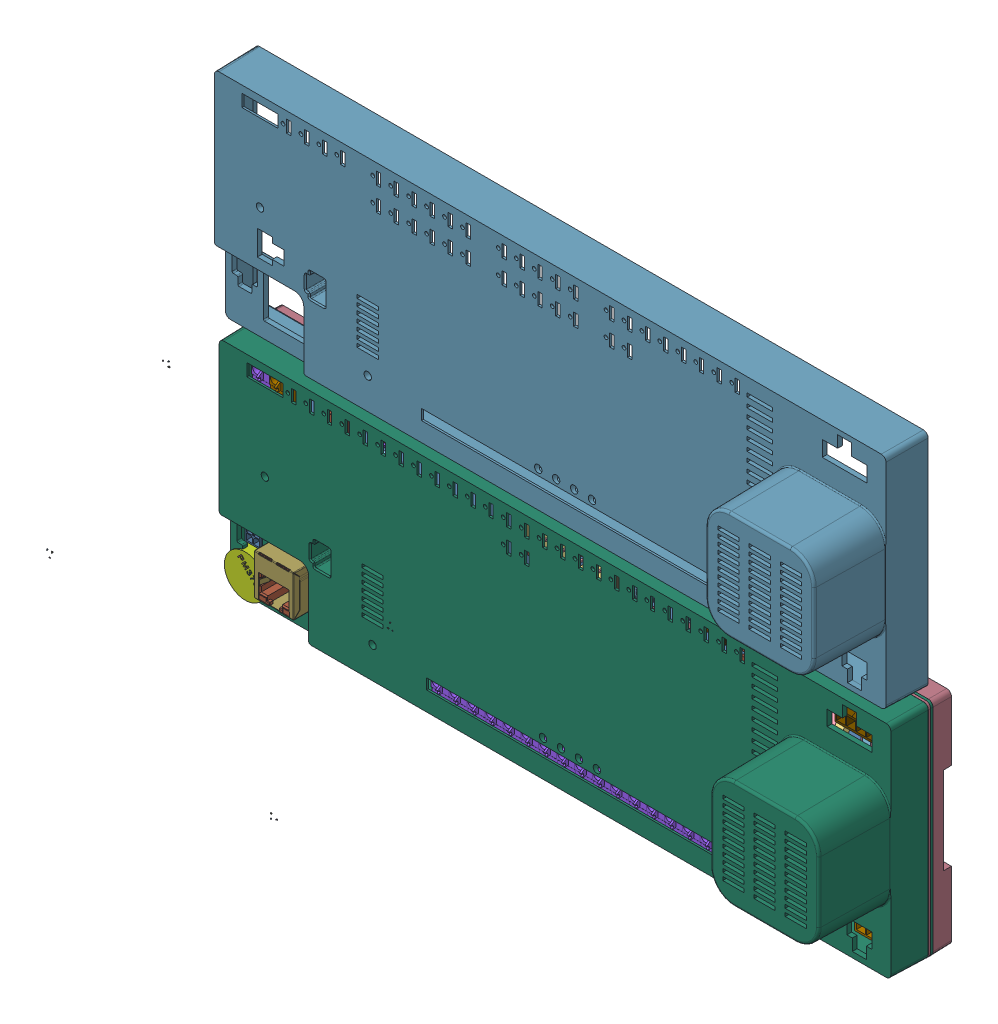
SolidWorks assembly _SC944D, configuration Default. Lengths in mm. (continued)
Components (placement in the parent): (continued)
- T58-1: T58 [Default] at origin size (130.97 33.9 23.48)
  - SW3dPS-transistor_SOT233-1: SW3dPS-transistor_SOT233 [Default] at (127.5968 31.0332 -21.9) x (-1 0 0) z (0 1 0) size (2.9 1.1 1.6)
  - SW3dPS-transistor_SOT233_1-1: SW3dPS-transistor_SOT233_1 [Default] at (0.1276 0.031 -0.0219) x (-1 0 0) z (0 1 0) size (2.18 2.18 2.18)
  - SW3dPS-transistor_SOT233_2-1: SW3dPS-transistor_SOT233_2 [Default] at (0.0001 0 0) x (-1 0 0) z (0 1 0) size (2.18 2.18 2.18)
  - SW3dPS-transistor_SOT233_3-1: SW3dPS-transistor_SOT233_3 [Default] x (-1 0 0) z (0 1 0) size (2.18 2.18 2.18)
- T59-1: T59 [Default] at origin size (136.17 33.9 23.48)
  - SW3dPS-transistor_SOT233-1: SW3dPS-transistor_SOT233 [Default] at (132.8038 31.0332 -21.9) x (-1 0 0) z (0 1 0) size (2.9 1.1 1.6)
  - SW3dPS-transistor_SOT233_1-1: SW3dPS-transistor_SOT233_1 [Default] at (0.1328 0.031 -0.0219) x (-1 0 0) z (0 1 0) size (2.18 2.18 2.18)
  - SW3dPS-transistor_SOT233_2-1: SW3dPS-transistor_SOT233_2 [Default] at (0.0001 0 0) x (-1 0 0) z (0 1 0) size (2.18 2.18 2.18)
  - SW3dPS-transistor_SOT233_3-1: SW3dPS-transistor_SOT233_3 [Default] x (-1 0 0) z (0 1 0) size (2.18 2.18 2.18)
- T60-1: T60 [Default] at origin size (90.38 86.77 23.48)
  - SW3dPS-transistor_SOT233-1: SW3dPS-transistor_SOT233 [Default] at (86.9062 83.9018 -21.9) x (1 0 0) z (0 -1 0) size (2.9 1.1 1.6)
  - SW3dPS-transistor_SOT233_1-1: SW3dPS-transistor_SOT233_1 [Default] at (0.0869 0.0839 -0.0219) x (1 0 0) z (0 -1 0) size (2.18 2.18 2.18)
  - SW3dPS-transistor_SOT233_2-1: SW3dPS-transistor_SOT233_2 [Default] at (0.0001 0.0001 0) x (1 0 0) z (0 -1 0) size (2.18 2.18 2.18)
  - SW3dPS-transistor_SOT233_3-1: SW3dPS-transistor_SOT233_3 [Default] x (1 0 0) z (0 -1 0) size (2.18 2.18 2.18)
- T61-1: T61 [Default] at origin size (89.91 93.6 23.48)
  - SW3dPS-transistor_SOT233-1: SW3dPS-transistor_SOT233 [Default] at (86.4299 90.7281 -21.9) x (1 0 0) z (0 -1 0) size (2.9 1.1 1.6)
  - SW3dPS-transistor_SOT233_1-1: SW3dPS-transistor_SOT233_1 [Default] at (0.0864 0.0907 -0.0219) x (1 0 0) z (0 -1 0) size (2.18 2.18 2.18)
  - SW3dPS-transistor_SOT233_2-1: SW3dPS-transistor_SOT233_2 [Default] at (0.0001 0.0001 0) x (1 0 0) z (0 -1 0) size (2.18 2.18 2.18)
  - SW3dPS-transistor_SOT233_3-1: SW3dPS-transistor_SOT233_3 [Default] x (1 0 0) z (0 -1 0) size (2.18 2.18 2.18)
- T62-1: T62 [Default] at origin size (81.97 92.65 23.48)
  - SW3dPS-transistor_SOT233-1: SW3dPS-transistor_SOT233 [Default] at (78.4924 89.7756 -21.9) x (1 0 0) z (0 -1 0) size (2.9 1.1 1.6)
  - SW3dPS-transistor_SOT233_1-1: SW3dPS-transistor_SOT233_1 [Default] at (0.0785 0.0898 -0.0219) x (1 0 0) z (0 -1 0) size (2.18 2.18 2.18)
  - SW3dPS-transistor_SOT233_2-1: SW3dPS-transistor_SOT233_2 [Default] at (0.0001 0.0001 0) x (1 0 0) z (0 -1 0) size (2.18 2.18 2.18)
  - SW3dPS-transistor_SOT233_3-1: SW3dPS-transistor_SOT233_3 [Default] x (1 0 0) z (0 -1 0) size (2.18 2.18 2.18)
- T63-1: T63 [Default] at origin size (84.51 85.66 23.48)
  - SW3dPS-transistor_SOT233-1: SW3dPS-transistor_SOT233 [Default] at (81.0324 82.7906 -21.9) x (1 0 0) z (0 -1 0) size (2.9 1.1 1.6)
  - SW3dPS-transistor_SOT233_1-1: SW3dPS-transistor_SOT233_1 [Default] at (0.081 0.0828 -0.0219) x (1 0 0) z (0 -1 0) size (2.18 2.18 2.18)
  - SW3dPS-transistor_SOT233_2-1: SW3dPS-transistor_SOT233_2 [Default] at (0.0001 0.0001 0) x (1 0 0) z (0 -1 0) size (2.18 2.18 2.18)
  - SW3dPS-transistor_SOT233_3-1: SW3dPS-transistor_SOT233_3 [Default] x (1 0 0) z (0 -1 0) size (2.18 2.18 2.18)
- T64-1: T64 [Default] at origin size (158.8 53.28 23.48)
  - SW3dPS-transistor_SOT233-1: SW3dPS-transistor_SOT233 [Default] at (155.3274 50.4056 -21.9) x (1 0 0) z (0 -1 0) size (2.9 1.1 1.6)
  - SW3dPS-transistor_SOT233_1-1: SW3dPS-transistor_SOT233_1 [Default] at (0.1553 0.0504 -0.0219) x (1 0 0) z (0 -1 0) size (2.18 2.18 2.18)
  - SW3dPS-transistor_SOT233_2-1: SW3dPS-transistor_SOT233_2 [Default] at (0.0002 0.0001 0) x (1 0 0) z (0 -1 0) size (2.18 2.18 2.18)
  - SW3dPS-transistor_SOT233_3-1: SW3dPS-transistor_SOT233_3 [Default] x (1 0 0) z (0 -1 0) size (2.18 2.18 2.18)
- T65-1: T65 [Default] at origin size (32.85 79.63 23.48)
  - SW3dPS-transistor_SOT233-1: SW3dPS-transistor_SOT233 [Default] at (29.9742 76.1522 -21.9) x (0 1 0) z (1 0 0) size (2.9 1.1 1.6)
  - SW3dPS-transistor_SOT233_1-1: SW3dPS-transistor_SOT233_1 [Default] at (0.03 0.0762 -0.0219) x (0 1 0) z (1 0 0) size (2.18 2.18 2.18)
  - SW3dPS-transistor_SOT233_2-1: SW3dPS-transistor_SOT233_2 [Default] at (0 0.0001 0) x (0 1 0) z (1 0 0) size (2.18 2.18 2.18)
  - SW3dPS-transistor_SOT233_3-1: SW3dPS-transistor_SOT233_3 [Default] x (0 1 0) z (1 0 0) size (2.18 2.18 2.18)
- T66-1: T66 [Default] at origin size (165.61 55.37 23.48)
  - SW3dPS-transistor_SOT233-1: SW3dPS-transistor_SOT233 [Default] at (162.2678 52.4962 -21.9) x (-1 0 0) z (0 1 0) size (2.9 1.1 1.6)
  - SW3dPS-transistor_SOT233_1-1: SW3dPS-transistor_SOT233_1 [Default] at (0.1623 0.0525 -0.0219) x (-1 0 0) z (0 1 0) size (2.18 2.18 2.18)
  - SW3dPS-transistor_SOT233_2-1: SW3dPS-transistor_SOT233_2 [Default] at (0.0002 0.0001 0) x (-1 0 0) z (0 1 0) size (2.18 2.18 2.18)
  - SW3dPS-transistor_SOT233_3-1: SW3dPS-transistor_SOT233_3 [Default] x (-1 0 0) z (0 1 0) size (2.18 2.18 2.18)
- U1-1: U1 [Default] at origin size (6.4 5 1.08)
  - SW3dPS-TSSOP-16-1: SW3dPS-TSSOP-16 [Default] at (33.8137 57.7851 0) x (0 1 0) z (0 0 1) size (5 6.4 1.08)
- U2-1: U2 [Default] at origin size (3 3 1.35)
  - User_Library-SOT23-6-1: User_Library-SOT23-6 [Default] at (72.8979 53.5939 0) x (-1 0 0) z (0 0 1) size (3 3 1.35)
- U3-1: U3 [Default] at origin size (9.19 5.08 4.7)
  - SOIC_pin_2-1: SOIC_pin_2 [Default] at (91.8173 23.0238 1) x (0 1 0) z (1 0 0) size (0.4 1.1 1.1)
  - SOIC_pin_2-2: SOIC_pin_2 [Default] at (88.8236 28.0938 1) x (0 -1 0) z (-1 0 0) size (0.4 1.1 1.1)
  - SOIC_pin_2-3: SOIC_pin_2 [Default] at (88.8236 30.6337 1) x (0 -1 0) z (-1 0 0) size (0.4 1.1 1.1)
  - SOIC_pin_2-4: SOIC_pin_2 [Default] at (91.8173 20.4838 1) x (0 1 0) z (1 0 0) size (0.4 1.1 1.1)
  - 1175074120-1: 1175074120 [Default] at (93.6466 25.5588 0) size (0.41 5.08 4.5)
    - Extruded-1: Extruded [Default] at origin size (0.41 5.08 4.5)
  - 1175073984-1: 1175073984 [Default] at (90.3287 25.5588 0) size (7.05 5.08 4.6)
    - Extruded_1-1: Extruded_1 [Default] at origin size (7.05 5.08 4.6)
  - 1173466944-1: 1173466944 [Default] at (92.2336 23.6538 4.6) x (0 1 0) z (0 0 1) size (0.4 0.4 0.1)
    - Cylinder-1: Cylinder [Default] at origin size (0.4 0.4 0.1)
- U4-1: U4 [Default] at origin size (19.5 9.8 14.1)
  - 1175074392-1: 1175074392 [Default] at (162.4959 50.1649 -1.6) size (0.5 0.5 1.6)
    - Extruded_2-1: Extruded_2 [Default] at origin size (0.5 0.5 1.6)
  - 1175074392-2: 1175074392 [Default] at (167.5759 50.1649 -1.6) size (0.5 0.5 1.6)
    - Extruded_2-1: Extruded_2 [Default] at origin size (0.5 0.5 1.6)
  - 1175074392-3: 1175074392 [Default] at (175.1959 50.1649 -1.6) size (0.5 0.5 1.6)
    - Extruded_2-1: Extruded_2 [Default] at origin size (0.5 0.5 1.6)
  - 1175074392-4: 1175074392 [Default] at (177.7359 50.1649 -1.6) size (0.5 0.5 1.6)
    - Extruded_2-1: Extruded_2 [Default] at origin size (0.5 0.5 1.6)
  - 1175074256-1: 1175074256 [Default] at (169.886 52.665 0) size (19.5 9.8 12.5)
    - Extruded_3-1: Extruded_3 [Default] at origin size (19.5 9.8 12.5)
- U5-1: U5 [Default] at origin size (2.02 2.1 0.95)
  - SW3dPS-SC70-6-1: SW3dPS-SC70-6 [Default] at (42.2275 56.4063 0.5) x (-1 0 0) z (0 1 0) size (2.02 0.95 2.1)
- U6-1: U6 [Default] at origin size (9.19 5.08 4.7)
  - SOIC_pin_2-1: SOIC_pin_2 [Default] at (91.765 35.7474 1) x (0 -1 0) z (-1 0 0) size (0.4 1.1 1.1)
  - SOIC_pin_2-2: SOIC_pin_2 [Default] at (94.7588 30.6774 1) x (0 1 0) z (1 0 0) size (0.4 1.1 1.1)
  - SOIC_pin_2-3: SOIC_pin_2 [Default] at (94.7588 28.1374 1) x (0 1 0) z (1 0 0) size (0.4 1.1 1.1)
  - SOIC_pin_2-4: SOIC_pin_2 [Default] at (91.765 38.2874 1) x (0 -1 0) z (-1 0 0) size (0.4 1.1 1.1)
  - 1175074120-1: 1175074120 [Default] at (89.9357 33.2124 0) size (0.41 5.08 4.5)
    - Extruded-1: Extruded [Default] at origin size (0.41 5.08 4.5)
  - 1175073984-1: 1175073984 [Default] at (93.2536 33.2123 0) size (7.05 5.08 4.6)
    - Extruded_1-1: Extruded_1 [Default] at origin size (7.05 5.08 4.6)
  - 1173467200-1: 1173467200 [Default] at (91.3487 35.1173 4.6) x (0 -1 0) z (0 0 1) size (0.4 0.4 0.1)
    - Cylinder_1-1: Cylinder_1 [Default] at origin size (0.4 0.4 0.1)
- U7-1: U7 [Default] at origin size (9.19 5.08 4.7)
  - SOIC_pin_2-1: SOIC_pin_2 [Default] at (91.765 42.0974 1) x (0 -1 0) z (-1 0 0) size (0.4 1.1 1.1)
  - SOIC_pin_2-2: SOIC_pin_2 [Default] at (94.7588 37.0274 1) x (0 1 0) z (1 0 0) size (0.4 1.1 1.1)
  - SOIC_pin_2-3: SOIC_pin_2 [Default] at (94.7588 34.4874 1) x (0 1 0) z (1 0 0) size (0.4 1.1 1.1)
  - SOIC_pin_2-4: SOIC_pin_2 [Default] at (91.765 44.6374 1) x (0 -1 0) z (-1 0 0) size (0.4 1.1 1.1)
  - 1175074120-1: 1175074120 [Default] at (89.9357 39.5624 0) size (0.41 5.08 4.5)
    - Extruded-1: Extruded [Default] at origin size (0.41 5.08 4.5)
  - 1175073984-1: 1175073984 [Default] at (93.2536 39.5623 0) size (7.05 5.08 4.6)
    - Extruded_1-1: Extruded_1 [Default] at origin size (7.05 5.08 4.6)
  - 1173467200-1: 1173467200 [Default] at (91.3487 41.4673 4.6) x (0 -1 0) z (0 0 1) size (0.4 0.4 0.1)
    - Cylinder_1-1: Cylinder_1 [Default] at origin size (0.4 0.4 0.1)
- U8-1: U8 [Default] at origin size (2.3 2.1 1)
  - User_Library-sot353-1: User_Library-sot353 [Default] at (38.093 43.3728 0) x (0 1 0) z (0 0 1) size (2.1 2.3 1)
- U9-1: U9 [Default] at origin size (3 3 1.35)
  - User_Library-SOT23-6-1: User_Library-SOT23-6 [Default] at (59.0551 45.8788 0) x (1 0 0) z (0 0 1) size (3 3 1.35)
- U10-1: U10 [Default] at origin size (22 22 1.6)
  - User_Library-LQFP144-1: User_Library-LQFP144 [Default] at (60.232 23.8429 0) x (-1 0 0) z (0 1 0) size (22 1.6 22)
    - User_Library-LQFP144_Assu_Fuss_LQFP144-1: User_Library-LQFP144_Assu_Fuss_LQFP144 [Default] at (10 0 0) size (1 0.89 17.72)
      - User_Library-LQFP144_Fuss_LQFP144-1: User_Library-LQFP144_Fuss_LQFP144 [Default] at (0 0 3.25) size (1 0.89 0.22)
      - User_Library-LQFP144_Fuss_LQFP144-2: User_Library-LQFP144_Fuss_LQFP144 [Default] at (0 0 -5.75) size (1 0.89 0.22)
      - User_Library-LQFP144_Fuss_LQFP144-3: User_Library-LQFP144_Fuss_LQFP144 [Default] at (0 0 -3.75) size (1 0.89 0.22)
      - User_Library-LQFP144_Fuss_LQFP144-4: User_Library-LQFP144_Fuss_LQFP144 [Default] at (0 0 -0.25) size (1 0.89 0.22)
      - User_Library-LQFP144_Fuss_LQFP144-5: User_Library-LQFP144_Fuss_LQFP144 [Default] at (0 0 -5.25) size (1 0.89 0.22)
      - User_Library-LQFP144_Fuss_LQFP144-6: User_Library-LQFP144_Fuss_LQFP144 [Default] at (0 0 -8.25) size (1 0.89 0.22)
      - User_Library-LQFP144_Fuss_LQFP144-7: User_Library-LQFP144_Fuss_LQFP144 [Default] at (0 0 -0.25) size (1 0.89 0.22)
      - User_Library-LQFP144_Fuss_LQFP144-8: User_Library-LQFP144_Fuss_LQFP144 [Default] at (0 0 -3.75) size (1 0.89 0.22)
      - User_Library-LQFP144_Fuss_LQFP144-9: User_Library-LQFP144_Fuss_LQFP144 [Default] at (0 0 -0.25) size (1 0.89 0.22)
      - User_Library-LQFP144_Fuss_LQFP144-10: User_Library-LQFP144_Fuss_LQFP144 [Default] at (0 0 6.75) size (1 0.89 0.22)
      - User_Library-LQFP144_Fuss_LQFP144-11: User_Library-LQFP144_Fuss_LQFP144 [Default] at (0 0 -3.75) size (1 0.89 0.22)
      - User_Library-LQFP144_Fuss_LQFP144-12: User_Library-LQFP144_Fuss_LQFP144 [Default] at (0 0 4.25) size (1 0.89 0.22)
      - User_Library-LQFP144_Fuss_LQFP144-13: User_Library-LQFP144_Fuss_LQFP144 [Default] at (0 0 0.75) size (1 0.89 0.22)
      - User_Library-LQFP144_Fuss_LQFP144-14: User_Library-LQFP144_Fuss_LQFP144 [Default] at (0 0 7.75) size (1 0.89 0.22)
      - User_Library-LQFP144_Fuss_LQFP144-15: User_Library-LQFP144_Fuss_LQFP144 [Default] at (0 0 1.75) size (1 0.89 0.22)
      - User_Library-LQFP144_Fuss_LQFP144-16: User_Library-LQFP144_Fuss_LQFP144 [Default] at (0 0 -2.25) size (1 0.89 0.22)
      - User_Library-LQFP144_Fuss_LQFP144-17: User_Library-LQFP144_Fuss_LQFP144 [Default] at (0 0 -2.75) size (1 0.89 0.22)
      - User_Library-LQFP144_Fuss_LQFP144-18: User_Library-LQFP144_Fuss_LQFP144 [Default] at (0 0 -4.25) size (1 0.89 0.22)
      - User_Library-LQFP144_Fuss_LQFP144-19: User_Library-LQFP144_Fuss_LQFP144 [Default] at (0 0 3.25) size (1 0.89 0.22)
      - User_Library-LQFP144_Fuss_LQFP144-20: User_Library-LQFP144_Fuss_LQFP144 [Default] at (0 0 -1.75) size (1 0.89 0.22)
      - User_Library-LQFP144_Fuss_LQFP144-21: User_Library-LQFP144_Fuss_LQFP144 [Default] at (0 0 -1.75) size (1 0.89 0.22)
      - User_Library-LQFP144_Fuss_LQFP144-22: User_Library-LQFP144_Fuss_LQFP144 [Default] at (0 0 2.75) size (1 0.89 0.22)
      - User_Library-LQFP144_Fuss_LQFP144-23: User_Library-LQFP144_Fuss_LQFP144 [Default] at (0 0 -2.75) size (1 0.89 0.22)
      - User_Library-LQFP144_Fuss_LQFP144-24: User_Library-LQFP144_Fuss_LQFP144 [Default] at (0 0 -3.75) size (1 0.89 0.22)
      - User_Library-LQFP144_Fuss_LQFP144-25: User_Library-LQFP144_Fuss_LQFP144 [Default] at (0 0 -5.75) size (1 0.89 0.22)
      - User_Library-LQFP144_Fuss_LQFP144-26: User_Library-LQFP144_Fuss_LQFP144 [Default] at (0 0 0.75) size (1 0.89 0.22)
      - User_Library-LQFP144_Fuss_LQFP144-27: User_Library-LQFP144_Fuss_LQFP144 [Default] at (0 0 -6.25) size (1 0.89 0.22)
      - User_Library-LQFP144_Fuss_LQFP144-28: User_Library-LQFP144_Fuss_LQFP144 [Default] at (0 0 -2.75) size (1 0.89 0.22)
      - User_Library-LQFP144_Fuss_LQFP144-29: User_Library-LQFP144_Fuss_LQFP144 [Default] at (0 0 1.25) size (1 0.89 0.22)
      - User_Library-LQFP144_Fuss_LQFP144-30: User_Library-LQFP144_Fuss_LQFP144 [Default] at (0 0 -0.25) size (1 0.89 0.22)
      - User_Library-LQFP144_Fuss_LQFP144-31: User_Library-LQFP144_Fuss_LQFP144 [Default] at (0 0 -1.25) size (1 0.89 0.22)
      - User_Library-LQFP144_Fuss_LQFP144-32: User_Library-LQFP144_Fuss_LQFP144 [Default] at (0 0 5.25) size (1 0.89 0.22)
      - User_Library-LQFP144_Fuss_LQFP144-33: User_Library-LQFP144_Fuss_LQFP144 [Default] at (0 0 8.25) size (1 0.89 0.22)
      - User_Library-LQFP144_Fuss_LQFP144-34: User_Library-LQFP144_Fuss_LQFP144 [Default] at (0 0 -6.25) size (1 0.89 0.22)
      - User_Library-LQFP144_Fuss_LQFP144-35: User_Library-LQFP144_Fuss_LQFP144 [Default] at (0 0 -0.75) size (1 0.89 0.22)
      - User_Library-LQFP144_Fuss_LQFP144-36: User_Library-LQFP144_Fuss_LQFP144 [Default] at (0 0 -8.75) size (1 0.89 0.22)
      - User_Library-LQFP144_Fuss_LQFP144-37: User_Library-LQFP144_Fuss_LQFP144 [Default] at (0 0 -1.25) size (1 0.89 0.22)
      - User_Library-LQFP144_Fuss_LQFP144-38: User_Library-LQFP144_Fuss_LQFP144 [Default] at (0 0 -1.25) size (1 0.89 0.22)
      - User_Library-LQFP144_Fuss_LQFP144-39: User_Library-LQFP144_Fuss_LQFP144 [Default] at (0 0 -2.75) size (1 0.89 0.22)
      - User_Library-LQFP144_Fuss_LQFP144-40: User_Library-LQFP144_Fuss_LQFP144 [Default] at (0 0 -2.75) size (1 0.89 0.22)
      - User_Library-LQFP144_Fuss_LQFP144-41: User_Library-LQFP144_Fuss_LQFP144 [Default] at (0 0 2.25) size (1 0.89 0.22)
      - User_Library-LQFP144_Fuss_LQFP144-42: User_Library-LQFP144_Fuss_LQFP144 [Default] at (0 0 3.75) size (1 0.89 0.22)
      - User_Library-LQFP144_Fuss_LQFP144-43: User_Library-LQFP144_Fuss_LQFP144 [Default] at (0 0 0.75) size (1 0.89 0.22)
      - User_Library-LQFP144_Fuss_LQFP144-44: User_Library-LQFP144_Fuss_LQFP144 [Default] at (0 0 0.75) size (1 0.89 0.22)
      - User_Library-LQFP144_Fuss_LQFP144-45: User_Library-LQFP144_Fuss_LQFP144 [Default] at (0 0 1.25) size (1 0.89 0.22)
      - User_Library-LQFP144_Fuss_LQFP144-46: User_Library-LQFP144_Fuss_LQFP144 [Default] at (0 0 1.75) size (1 0.89 0.22)
      - User_Library-LQFP144_Fuss_LQFP144-47: User_Library-LQFP144_Fuss_LQFP144 [Default] at (0 0 3.25) size (1 0.89 0.22)
      - User_Library-LQFP144_Fuss_LQFP144-48: User_Library-LQFP144_Fuss_LQFP144 [Default] at (0 0 -3.25) size (1 0.89 0.22)
      - User_Library-LQFP144_Fuss_LQFP144-49: User_Library-LQFP144_Fuss_LQFP144 [Default] at (0 0 5.75) size (1 0.89 0.22)
      - User_Library-LQFP144_Fuss_LQFP144-50: User_Library-LQFP144_Fuss_LQFP144 [Default] at (0 0 4.25) size (1 0.89 0.22)
      - User_Library-LQFP144_Fuss_LQFP144-51: User_Library-LQFP144_Fuss_LQFP144 [Default] at (0 0 3.25) size (1 0.89 0.22)
      - User_Library-LQFP144_Fuss_LQFP144-52: User_Library-LQFP144_Fuss_LQFP144 [Default] at (0 0 6.25) size (1 0.89 0.22)
      - User_Library-LQFP144_Fuss_LQFP144-53: User_Library-LQFP144_Fuss_LQFP144 [Default] at (0 0 -5.25) size (1 0.89 0.22)
      - User_Library-LQFP144_Fuss_LQFP144-54: User_Library-LQFP144_Fuss_LQFP144 [Default] at (0 0 -6.75) size (1 0.89 0.22)
      - User_Library-LQFP144_Fuss_LQFP144-55: User_Library-LQFP144_Fuss_LQFP144 [Default] at (0 0 -0.75) size (1 0.89 0.22)
      - User_Library-LQFP144_Fuss_LQFP144-56: User_Library-LQFP144_Fuss_LQFP144 [Default] at (0 0 1.75) size (1 0.89 0.22)
      - User_Library-LQFP144_Fuss_LQFP144-57: User_Library-LQFP144_Fuss_LQFP144 [Default] at (0 0 -3.25) size (1 0.89 0.22)
      - User_Library-LQFP144_Fuss_LQFP144-58: User_Library-LQFP144_Fuss_LQFP144 [Default] at (0 0 -4.25) size (1 0.89 0.22)
      - User_Library-LQFP144_Fuss_LQFP144-59: User_Library-LQFP144_Fuss_LQFP144 [Default] at (0 0 -5.25) size (1 0.89 0.22)
      - User_Library-LQFP144_Fuss_LQFP144-60: User_Library-LQFP144_Fuss_LQFP144 [Default] at (0 0 -1.25) size (1 0.89 0.22)
      - User_Library-LQFP144_Fuss_LQFP144-61: User_Library-LQFP144_Fuss_LQFP144 [Default] at (0 0 -0.75) size (1 0.89 0.22)
      - User_Library-LQFP144_Fuss_LQFP144-62: User_Library-LQFP144_Fuss_LQFP144 [Default] at (0 0 -6.25) size (1 0.89 0.22)
      - User_Library-LQFP144_Fuss_LQFP144-63: User_Library-LQFP144_Fuss_LQFP144 [Default] at (0 0 4.75) size (1 0.89 0.22)
      - User_Library-LQFP144_Fuss_LQFP144-64: User_Library-LQFP144_Fuss_LQFP144 [Default] at (0 0 3.25) size (1 0.89 0.22)
      - User_Library-LQFP144_Fuss_LQFP144-65: User_Library-LQFP144_Fuss_LQFP144 [Default] at (0 0 4.25) size (1 0.89 0.22)
      - User_Library-LQFP144_Fuss_LQFP144-66: User_Library-LQFP144_Fuss_LQFP144 [Default] at (0 0 0.25) size (1 0.89 0.22)
      - User_Library-LQFP144_Fuss_LQFP144-67: User_Library-LQFP144_Fuss_LQFP144 [Default] at (0 0 4.25) size (1 0.89 0.22)
      - User_Library-LQFP144_Fuss_LQFP144-68: User_Library-LQFP144_Fuss_LQFP144 [Default] at (0 0 6.75) size (1 0.89 0.22)
      - User_Library-LQFP144_Fuss_LQFP144-69: User_Library-LQFP144_Fuss_LQFP144 [Default] at (0 0 0.25) size (1 0.89 0.22)
      - User_Library-LQFP144_Fuss_LQFP144-70: User_Library-LQFP144_Fuss_LQFP144 [Default] at (0 0 0.25) size (1 0.89 0.22)
      - User_Library-LQFP144_Fuss_LQFP144-71: User_Library-LQFP144_Fuss_LQFP144 [Default] at (0 0 -1.25) size (1 0.89 0.22)
      - User_Library-LQFP144_Fuss_LQFP144-72: User_Library-LQFP144_Fuss_LQFP144 [Default] at (0 0 -3.75) size (1 0.89 0.22)
      - User_Library-LQFP144_Fuss_LQFP144-73: User_Library-LQFP144_Fuss_LQFP144 [Default] at (0 0 -0.25) size (1 0.89 0.22)
      - User_Library-LQFP144_Fuss_LQFP144-74: User_Library-LQFP144_Fuss_LQFP144 [Default] at (0 0 1.25) size (1 0.89 0.22)
      - User_Library-LQFP144_Fuss_LQFP144-75: User_Library-LQFP144_Fuss_LQFP144 [Default] at (0 0 0.75) size (1 0.89 0.22)
      - User_Library-LQFP144_Fuss_LQFP144-76: User_Library-LQFP144_Fuss_LQFP144 [Default] at (0 0 -7.75) size (1 0.89 0.22)
      - User_Library-LQFP144_Fuss_LQFP144-77: User_Library-LQFP144_Fuss_LQFP144 [Default] at (0 0 -3.25) size (1 0.89 0.22)
      - User_Library-LQFP144_Fuss_LQFP144-78: User_Library-LQFP144_Fuss_LQFP144 [Default] at (0 0 2.75) size (1 0.89 0.22)
      - User_Library-LQFP144_Fuss_LQFP144-79: User_Library-LQFP144_Fuss_LQFP144 [Default] at (0 0 4.75) size (1 0.89 0.22)
      - User_Library-LQFP144_Fuss_LQFP144-80: User_Library-LQFP144_Fuss_LQFP144 [Default] at (0 0 -7.25) size (1 0.89 0.22)
      - User_Library-LQFP144_Fuss_LQFP144-81: User_Library-LQFP144_Fuss_LQFP144 [Default] at (0 0 0.75) size (1 0.89 0.22)
      - User_Library-LQFP144_Fuss_LQFP144-82: User_Library-LQFP144_Fuss_LQFP144 [Default] at (0 0 0.75) size (1 0.89 0.22)
      - User_Library-LQFP144_Fuss_LQFP144-83: User_Library-LQFP144_Fuss_LQFP144 [Default] at (0 0 -0.75) size (1 0.89 0.22)
      - User_Library-LQFP144_Fuss_LQFP144-84: User_Library-LQFP144_Fuss_LQFP144 [Default] at (0 0 6.75) size (1 0.89 0.22)
      - User_Library-LQFP144_Fuss_LQFP144-85: User_Library-LQFP144_Fuss_LQFP144 [Default] at (0 0 -3.25) size (1 0.89 0.22)
      - User_Library-LQFP144_Fuss_LQFP144-86: User_Library-LQFP144_Fuss_LQFP144 [Default] at (0 0 3.75) size (1 0.89 0.22)
      - User_Library-LQFP144_Fuss_LQFP144-87: User_Library-LQFP144_Fuss_LQFP144 [Default] at (0 0 -0.75) size (1 0.89 0.22)
      - User_Library-LQFP144_Fuss_LQFP144-88: User_Library-LQFP144_Fuss_LQFP144 [Default] at (0 0 -1.75) size (1 0.89 0.22)
      - User_Library-LQFP144_Fuss_LQFP144-89: User_Library-LQFP144_Fuss_LQFP144 [Default] at (0 0 7.25) size (1 0.89 0.22)
      - User_Library-LQFP144_Fuss_LQFP144-90: User_Library-LQFP144_Fuss_LQFP144 [Default] at (0 0 0.75) size (1 0.89 0.22)
      - User_Library-LQFP144_Fuss_LQFP144-91: User_Library-LQFP144_Fuss_LQFP144 [Default] at (0 0 0.25) size (1 0.89 0.22)
      - User_Library-LQFP144_Fuss_LQFP144-92: User_Library-LQFP144_Fuss_LQFP144 [Default] at (0 0 0.25) size (1 0.89 0.22)
      - User_Library-LQFP144_Fuss_LQFP144-93: User_Library-LQFP144_Fuss_LQFP144 [Default] at (0 0 0.25) size (1 0.89 0.22)
      - User_Library-LQFP144_Fuss_LQFP144-94: User_Library-LQFP144_Fuss_LQFP144 [Default] at (0 0 1.75) size (1 0.89 0.22)
      - User_Library-LQFP144_Fuss_LQFP144-95: User_Library-LQFP144_Fuss_LQFP144 [Default] at (0 0 3.25) size (1 0.89 0.22)
      - User_Library-LQFP144_Fuss_LQFP144-96: User_Library-LQFP144_Fuss_LQFP144 [Default] at (0 0 -2.75) size (1 0.89 0.22)
      - User_Library-LQFP144_Fuss_LQFP144-97: User_Library-LQFP144_Fuss_LQFP144 [Default] at (0 0 -1.75) size (1 0.89 0.22)
      - User_Library-LQFP144_Fuss_LQFP144-98: User_Library-LQFP144_Fuss_LQFP144 [Default] at (0 0 4.75) size (1 0.89 0.22)
      - User_Library-LQFP144_Fuss_LQFP144-99: User_Library-LQFP144_Fuss_LQFP144 [Default] at (0 0 1.25) size (1 0.89 0.22)
      - User_Library-LQFP144_Fuss_LQFP144-100: User_Library-LQFP144_Fuss_LQFP144 [Default] at (0 0 4.75) size (1 0.89 0.22)
      - User_Library-LQFP144_Fuss_LQFP144-101: User_Library-LQFP144_Fuss_LQFP144 [Default] at (0 0 2.25) size (1 0.89 0.22)
      - User_Library-LQFP144_Fuss_LQFP144-102: User_Library-LQFP144_Fuss_LQFP144 [Default] at (0 0 2.25) size (1 0.89 0.22)
      - User_Library-LQFP144_Fuss_LQFP144-103: User_Library-LQFP144_Fuss_LQFP144 [Default] at (0 0 -2.75) size (1 0.89 0.22)
      - User_Library-LQFP144_Fuss_LQFP144-104: User_Library-LQFP144_Fuss_LQFP144 [Default] at (0 0 1.75) size (1 0.89 0.22)
      - User_Library-LQFP144_Fuss_LQFP144-105: User_Library-LQFP144_Fuss_LQFP144 [Default] at (0 0 7.25) size (1 0.89 0.22)
      - User_Library-LQFP144_Fuss_LQFP144-106: User_Library-LQFP144_Fuss_LQFP144 [Default] at (0 0 4.25) size (1 0.89 0.22)
      - User_Library-LQFP144_Fuss_LQFP144-107: User_Library-LQFP144_Fuss_LQFP144 [Default] at (0 0 7.75) size (1 0.89 0.22)
      - User_Library-LQFP144_Fuss_LQFP144-108: User_Library-LQFP144_Fuss_LQFP144 [Default] at (0 0 4.25) size (1 0.89 0.22)
      - User_Library-LQFP144_Fuss_LQFP144-109: User_Library-LQFP144_Fuss_LQFP144 [Default] at (0 0 7.25) size (1 0.89 0.22)
      - User_Library-LQFP144_Fuss_LQFP144-110: User_Library-LQFP144_Fuss_LQFP144 [Default] at (0 0 1.25) size (1 0.89 0.22)
      - User_Library-LQFP144_Fuss_LQFP144-111: User_Library-LQFP144_Fuss_LQFP144 [Default] at (0 0 7.25) size (1 0.89 0.22)
      - User_Library-LQFP144_Fuss_LQFP144-112: User_Library-LQFP144_Fuss_LQFP144 [Default] at (0 0 5.25) size (1 0.89 0.22)
      - User_Library-LQFP144_Fuss_LQFP144-113: User_Library-LQFP144_Fuss_LQFP144 [Default] at (0 0 6.75) size (1 0.89 0.22)
      - User_Library-LQFP144_Fuss_LQFP144-114: User_Library-LQFP144_Fuss_LQFP144 [Default] at (0 0 -6.25) size (1 0.89 0.22)
      - User_Library-LQFP144_Fuss_LQFP144-115: User_Library-LQFP144_Fuss_LQFP144 [Default] at (0 0 -0.25) size (1 0.89 0.22)
      - User_Library-LQFP144_Fuss_LQFP144-116: User_Library-LQFP144_Fuss_LQFP144 [Default] at (0 0 0.25) size (1 0.89 0.22)
      - User_Library-LQFP144_Fuss_LQFP144-117: User_Library-LQFP144_Fuss_LQFP144 [Default] at (0 0 8.25) size (1 0.89 0.22)
      - User_Library-LQFP144_Fuss_LQFP144-118: User_Library-LQFP144_Fuss_LQFP144 [Default] at (0 0 -4.75) size (1 0.89 0.22)
      - User_Library-LQFP144_Fuss_LQFP144-119: User_Library-LQFP144_Fuss_LQFP144 [Default] at (0 0 -2.25) size (1 0.89 0.22)
      - User_Library-LQFP144_Fuss_LQFP144-120: User_Library-LQFP144_Fuss_LQFP144 [Default] at (0 0 -6.75) size (1 0.89 0.22)
      - User_Library-LQFP144_Fuss_LQFP144-121: User_Library-LQFP144_Fuss_LQFP144 [Default] at (0 0 -1.75) size (1 0.89 0.22)
      - User_Library-LQFP144_Fuss_LQFP144-122: User_Library-LQFP144_Fuss_LQFP144 [Default] at (0 0 -7.25) size (1 0.89 0.22)
      - User_Library-LQFP144_Fuss_LQFP144-123: User_Library-LQFP144_Fuss_LQFP144 [Default] at (0 0 -5.25) size (1 0.89 0.22)
      - User_Library-LQFP144_Fuss_LQFP144-124: User_Library-LQFP144_Fuss_LQFP144 [Default] at (0 0 -5.75) size (1 0.89 0.22)
      - User_Library-LQFP144_Fuss_LQFP144-125: User_Library-LQFP144_Fuss_LQFP144 [Default] at (0 0 2.75) size (1 0.89 0.22)
      - User_Library-LQFP144_Fuss_LQFP144-126: User_Library-LQFP144_Fuss_LQFP144 [Default] at (0 0 1.75) size (1 0.89 0.22)
      - User_Library-LQFP144_Fuss_LQFP144-127: User_Library-LQFP144_Fuss_LQFP144 [Default] at (0 0 0.25) size (1 0.89 0.22)
      - User_Library-LQFP144_Fuss_LQFP144-128: User_Library-LQFP144_Fuss_LQFP144 [Default] at (0 0 -3.25) size (1 0.89 0.22)
      - User_Library-LQFP144_Fuss_LQFP144-129: User_Library-LQFP144_Fuss_LQFP144 [Default] at (0 0 3.25) size (1 0.89 0.22)
      - User_Library-LQFP144_Fuss_LQFP144-130: User_Library-LQFP144_Fuss_LQFP144 [Default] at (0 0 -2.75) size (1 0.89 0.22)
      - User_Library-LQFP144_Fuss_LQFP144-131: User_Library-LQFP144_Fuss_LQFP144 [Default] at (0 0 3.75) size (1 0.89 0.22)
      - User_Library-LQFP144_Fuss_LQFP144-132: User_Library-LQFP144_Fuss_LQFP144 [Default] at (0 0 0.25) size (1 0.89 0.22)
      - User_Library-LQFP144_Fuss_LQFP144-133: User_Library-LQFP144_Fuss_LQFP144 [Default] at (0 0 2.25) size (1 0.89 0.22)
      - User_Library-LQFP144_Fuss_LQFP144-134: User_Library-LQFP144_Fuss_LQFP144 [Default] at (0 0 -1.25) size (1 0.89 0.22)
      - User_Library-LQFP144_Fuss_LQFP144-135: User_Library-LQFP144_Fuss_LQFP144 [Default] at (0 0 -0.75) size (1 0.89 0.22)
      - User_Library-LQFP144_Fuss_LQFP144-136: User_Library-LQFP144_Fuss_LQFP144 [Default] at (0 0 -4.25) size (1 0.89 0.22)
      - User_Library-LQFP144_Fuss_LQFP144-137: User_Library-LQFP144_Fuss_LQFP144 [Default] at (0 0 1.75) size (1 0.89 0.22)
      - User_Library-LQFP144_Fuss_LQFP144-138: User_Library-LQFP144_Fuss_LQFP144 [Default] at (0 0 -1.25) size (1 0.89 0.22)
      - User_Library-LQFP144_Fuss_LQFP144-139: User_Library-LQFP144_Fuss_LQFP144 [Default] at (0 0 -1.75) size (1 0.89 0.22)
      - User_Library-LQFP144_Fuss_LQFP144-140: User_Library-LQFP144_Fuss_LQFP144 [Default] at (0 0 4.25) size (1 0.89 0.22)
      - User_Library-LQFP144_Fuss_LQFP144-141: User_Library-LQFP144_Fuss_LQFP144 [Default] at (0 0 -2.25) size (1 0.89 0.22)
      - User_Library-LQFP144_Fuss_LQFP144-142: User_Library-LQFP144_Fuss_LQFP144 [Default] at (0 0 5.25) size (1 0.89 0.22)
      - User_Library-LQFP144_Fuss_LQFP144-143: User_Library-LQFP144_Fuss_LQFP144 [Default] at (0 0 2.75) size (1 0.89 0.22)
      - User_Library-LQFP144_Fuss_LQFP144-144: User_Library-LQFP144_Fuss_LQFP144 [Default] at (0 0 -1.75) size (1 0.89 0.22)
      - User_Library-LQFP144_Fuss_LQFP144-145: User_Library-LQFP144_Fuss_LQFP144 [Default] at (0 0 -0.25) size (1 0.89 0.22)
      - User_Library-LQFP144_Fuss_LQFP144-146: User_Library-LQFP144_Fuss_LQFP144 [Default] at (0 0 0.75) size (1 0.89 0.22)
      - User_Library-LQFP144_Fuss_LQFP144-147: User_Library-LQFP144_Fuss_LQFP144 [Default] at (0 0 -0.25) size (1 0.89 0.22)
      - User_Library-LQFP144_Fuss_LQFP144-148: User_Library-LQFP144_Fuss_LQFP144 [Default] at (0 0 3.75) size (1 0.89 0.22)
      - User_Library-LQFP144_Fuss_LQFP144-149: User_Library-LQFP144_Fuss_LQFP144 [Default] at (0 0 2.75) size (1 0.89 0.22)
      - User_Library-LQFP144_Fuss_LQFP144-150: User_Library-LQFP144_Fuss_LQFP144 [Default] at (0 0 2.75) size (1 0.89 0.22)
      - User_Library-LQFP144_Fuss_LQFP144-151: User_Library-LQFP144_Fuss_LQFP144 [Default] at (0 0 6.25) size (1 0.89 0.22)
      - User_Library-LQFP144_Fuss_LQFP144-152: User_Library-LQFP144_Fuss_LQFP144 [Default] at (0 0 2.25) size (1 0.89 0.22)
      - User_Library-LQFP144_Fuss_LQFP144-153: User_Library-LQFP144_Fuss_LQFP144 [Default] at (0 0 -0.75) size (1 0.89 0.22)
      - User_Library-LQFP144_Fuss_LQFP144-154: User_Library-LQFP144_Fuss_LQFP144 [Default] at (0 0 -2.25) size (1 0.89 0.22)
      - User_Library-LQFP144_Fuss_LQFP144-155: User_Library-LQFP144_Fuss_LQFP144 [Default] at (0 0 -0.75) size (1 0.89 0.22)
      - User_Library-LQFP144_Fuss_LQFP144-156: User_Library-LQFP144_Fuss_LQFP144 [Default] at (0 0 -2.25) size (1 0.89 0.22)
      - User_Library-LQFP144_Fuss_LQFP144-157: User_Library-LQFP144_Fuss_LQFP144 [Default] at (0 0 -2.25) size (1 0.89 0.22)
      - User_Library-LQFP144_Fuss_LQFP144-158: User_Library-LQFP144_Fuss_LQFP144 [Default] at (0 0 0.75) size (1 0.89 0.22)
      - User_Library-LQFP144_Fuss_LQFP144-159: User_Library-LQFP144_Fuss_LQFP144 [Default] at (0 0 -4.25) size (1 0.89 0.22)
      - User_Library-LQFP144_Fuss_LQFP144-160: User_Library-LQFP144_Fuss_LQFP144 [Default] at (0 0 4.25) size (1 0.89 0.22)
      - User_Library-LQFP144_Fuss_LQFP144-161: User_Library-LQFP144_Fuss_LQFP144 [Default] at (0 0 1.25) size (1 0.89 0.22)
      - User_Library-LQFP144_Fuss_LQFP144-162: User_Library-LQFP144_Fuss_LQFP144 [Default] at (0 0 -0.25) size (1 0.89 0.22)
      - User_Library-LQFP144_Fuss_LQFP144-163: User_Library-LQFP144_Fuss_LQFP144 [Default] at (0 0 -4.25) size (1 0.89 0.22)
      - User_Library-LQFP144_Fuss_LQFP144-164: User_Library-LQFP144_Fuss_LQFP144 [Default] at (0 0 -1.25) size (1 0.89 0.22)
      - User_Library-LQFP144_Fuss_LQFP144-165: User_Library-LQFP144_Fuss_LQFP144 [Default] at (0 0 -8.25) size (1 0.89 0.22)
      - User_Library-LQFP144_Fuss_LQFP144-166: User_Library-LQFP144_Fuss_LQFP144 [Default] at (0 0 -3.25) size (1 0.89 0.22)
      - User_Library-LQFP144_Fuss_LQFP144-167: User_Library-LQFP144_Fuss_LQFP144 [Default] at (0 0 -4.75) size (1 0.89 0.22)
      - User_Library-LQFP144_Fuss_LQFP144-168: User_Library-LQFP144_Fuss_LQFP144 [Default] at (0 0 -2.25) size (1 0.89 0.22)
      - User_Library-LQFP144_Fuss_LQFP144-169: User_Library-LQFP144_Fuss_LQFP144 [Default] at (0 0 -1.25) size (1 0.89 0.22)
      - User_Library-LQFP144_Fuss_LQFP144-170: User_Library-LQFP144_Fuss_LQFP144 [Default] at (0 0 -7.25) size (1 0.89 0.22)
      - User_Library-LQFP144_Fuss_LQFP144-171: User_Library-LQFP144_Fuss_LQFP144 [Default] at (0 0 -4.25) size (1 0.89 0.22)
      - User_Library-LQFP144_Fuss_LQFP144-172: User_Library-LQFP144_Fuss_LQFP144 [Default] at (0 0 -4.25) size (1 0.89 0.22)
      - User_Library-LQFP144_Fuss_LQFP144-173: User_Library-LQFP144_Fuss_LQFP144 [Default] at (0 0 1.75) size (1 0.89 0.22)
      - User_Library-LQFP144_Fuss_LQFP144-174: User_Library-LQFP144_Fuss_LQFP144 [Default] at (0 0 0.25) size (1 0.89 0.22)
      - User_Library-LQFP144_Fuss_LQFP144-175: User_Library-LQFP144_Fuss_LQFP144 [Default] at (0 0 -0.75) size (1 0.89 0.22)
      - User_Library-LQFP144_Fuss_LQFP144-176: User_Library-LQFP144_Fuss_LQFP144 [Default] at (0 0 0.75) size (1 0.89 0.22)
      - User_Library-LQFP144_Fuss_LQFP144-177: User_Library-LQFP144_Fuss_LQFP144 [Default] at (0 0 1.75) size (1 0.89 0.22)
      - User_Library-LQFP144_Fuss_LQFP144-178: User_Library-LQFP144_Fuss_LQFP144 [Default] at (0 0 -0.75) size (1 0.89 0.22)
      - User_Library-LQFP144_Fuss_LQFP144-179: User_Library-LQFP144_Fuss_LQFP144 [Default] at (0 0 3.75) size (1 0.89 0.22)
      - User_Library-LQFP144_Fuss_LQFP144-180: User_Library-LQFP144_Fuss_LQFP144 [Default] at (0 0 4.75) size (1 0.89 0.22)
      - User_Library-LQFP144_Fuss_LQFP144-181: User_Library-LQFP144_Fuss_LQFP144 [Default] at (0 0 -0.75) size (1 0.89 0.22)
      - User_Library-LQFP144_Fuss_LQFP144-182: User_Library-LQFP144_Fuss_LQFP144 [Default] at (0 0 2.75) size (1 0.89 0.22)
      - User_Library-LQFP144_Fuss_LQFP144-183: User_Library-LQFP144_Fuss_LQFP144 [Default] at (0 0 -1.25) size (1 0.89 0.22)
      - User_Library-LQFP144_Fuss_LQFP144-184: User_Library-LQFP144_Fuss_LQFP144 [Default] at (0 0 2.75) size (1 0.89 0.22)
      - User_Library-LQFP144_Fuss_LQFP144-185: User_Library-LQFP144_Fuss_LQFP144 [Default] at (0 0 5.25) size (1 0.89 0.22)
      - User_Library-LQFP144_Fuss_LQFP144-186: User_Library-LQFP144_Fuss_LQFP144 [Default] at (0 0 -4.25) size (1 0.89 0.22)
      - User_Library-LQFP144_Fuss_LQFP144-187: User_Library-LQFP144_Fuss_LQFP144 [Default] at (0 0 -4.75) size (1 0.89 0.22)
      - User_Library-LQFP144_Fuss_LQFP144-188: User_Library-LQFP144_Fuss_LQFP144 [Default] at (0 0 -3.75) size (1 0.89 0.22)
      - User_Library-LQFP144_Fuss_LQFP144-189: User_Library-LQFP144_Fuss_LQFP144 [Default] at (0 0 -6.25) size (1 0.89 0.22)
      - User_Library-LQFP144_Fuss_LQFP144-190: User_Library-LQFP144_Fuss_LQFP144 [Default] at (0 0 0.75) size (1 0.89 0.22)
      - User_Library-LQFP144_Fuss_LQFP144-191: User_Library-LQFP144_Fuss_LQFP144 [Default] at (0 0 0.25) size (1 0.89 0.22)
      - User_Library-LQFP144_Fuss_LQFP144-192: User_Library-LQFP144_Fuss_LQFP144 [Default] at (0 0 -0.25) size (1 0.89 0.22)
      - User_Library-LQFP144_Fuss_LQFP144-193: User_Library-LQFP144_Fuss_LQFP144 [Default] at (0 0 -3.25) size (1 0.89 0.22)
      - User_Library-LQFP144_Fuss_LQFP144-194: User_Library-LQFP144_Fuss_LQFP144 [Default] at (0 0 1.75) size (1 0.89 0.22)
      - User_Library-LQFP144_Fuss_LQFP144-195: User_Library-LQFP144_Fuss_LQFP144 [Default] at (0 0 0.25) size (1 0.89 0.22)
      - User_Library-LQFP144_Fuss_LQFP144-196: User_Library-LQFP144_Fuss_LQFP144 [Default] at (0 0 5.25) size (1 0.89 0.22)
      - User_Library-LQFP144_Fuss_LQFP144-197: User_Library-LQFP144_Fuss_LQFP144 [Default] at (0 0 -1.75) size (1 0.89 0.22)
      - User_Library-LQFP144_Fuss_LQFP144-198: User_Library-LQFP144_Fuss_LQFP144 [Default] at (0 0 5.75) size (1 0.89 0.22)
      - User_Library-LQFP144_Fuss_LQFP144-199: User_Library-LQFP144_Fuss_LQFP144 [Default] at (0 0 5.75) size (1 0.89 0.22)
      - User_Library-LQFP144_Fuss_LQFP144-200: User_Library-LQFP144_Fuss_LQFP144 [Default] at (0 0 3.25) size (1 0.89 0.22)
      - User_Library-LQFP144_Fuss_LQFP144-201: User_Library-LQFP144_Fuss_LQFP144 [Default] at (0 0 0.25) size (1 0.89 0.22)
      - User_Library-LQFP144_Fuss_LQFP144-202: User_Library-LQFP144_Fuss_LQFP144 [Default] at (0 0 -1.75) size (1 0.89 0.22)
      - User_Library-LQFP144_Fuss_LQFP144-203: User_Library-LQFP144_Fuss_LQFP144 [Default] at (0 0 -5.75) size (1 0.89 0.22)
      - User_Library-LQFP144_Fuss_LQFP144-204: User_Library-LQFP144_Fuss_LQFP144 [Default] at (0 0 1.25) size (1 0.89 0.22)
      - User_Library-LQFP144_Fuss_LQFP144-205: User_Library-LQFP144_Fuss_LQFP144 [Default] at (0 0 2.25) size (1 0.89 0.22)
      - User_Library-LQFP144_Fuss_LQFP144-206: User_Library-LQFP144_Fuss_LQFP144 [Default] at (0 0 -1.25) size (1 0.89 0.22)
      - User_Library-LQFP144_Fuss_LQFP144-207: User_Library-LQFP144_Fuss_LQFP144 [Default] at (0 0 -1.25) size (1 0.89 0.22)
      - User_Library-LQFP144_Fuss_LQFP144-208: User_Library-LQFP144_Fuss_LQFP144 [Default] at (0 0 -0.25) size (1 0.89 0.22)
      - User_Library-LQFP144_Fuss_LQFP144-209: User_Library-LQFP144_Fuss_LQFP144 [Default] at (0 0 1.25) size (1 0.89 0.22)
      - User_Library-LQFP144_Fuss_LQFP144-210: User_Library-LQFP144_Fuss_LQFP144 [Default] at (0 0 6.25) size (1 0.89 0.22)
      - User_Library-LQFP144_Fuss_LQFP144-211: User_Library-LQFP144_Fuss_LQFP144 [Default] at (0 0 5.75) size (1 0.89 0.22)
      - User_Library-LQFP144_Fuss_LQFP144-212: User_Library-LQFP144_Fuss_LQFP144 [Default] at (0 0 1.25) size (1 0.89 0.22)
      - User_Library-LQFP144_Fuss_LQFP144-213: User_Library-LQFP144_Fuss_LQFP144 [Default] at (0 0 -0.25) size (1 0.89 0.22)
      - User_Library-LQFP144_Fuss_LQFP144-214: User_Library-LQFP144_Fuss_LQFP144 [Default] at (0 0 6.25) size (1 0.89 0.22)
      - User_Library-LQFP144_Fuss_LQFP144-215: User_Library-LQFP144_Fuss_LQFP144 [Default] at (0 0 -0.75) size (1 0.89 0.22)
      - User_Library-LQFP144_Fuss_LQFP144-216: User_Library-LQFP144_Fuss_LQFP144 [Default] at (0 0 5.25) size (1 0.89 0.22)
      - User_Library-LQFP144_Fuss_LQFP144-217: User_Library-LQFP144_Fuss_LQFP144 [Default] at (0 0 -2.25) size (1 0.89 0.22)
      - User_Library-LQFP144_Fuss_LQFP144-218: User_Library-LQFP144_Fuss_LQFP144 [Default] at (0 0 2.75) size (1 0.89 0.22)
      - User_Library-LQFP144_Fuss_LQFP144-219: User_Library-LQFP144_Fuss_LQFP144 [Default] at (0 0 -1.75) size (1 0.89 0.22)
      - User_Library-LQFP144_Fuss_LQFP144-220: User_Library-LQFP144_Fuss_LQFP144 [Default] at (0 0 -5.25) size (1 0.89 0.22)
      - User_Library-LQFP144_Fuss_LQFP144-221: User_Library-LQFP144_Fuss_LQFP144 [Default] at (0 0 1.25) size (1 0.89 0.22)
      - User_Library-LQFP144_Fuss_LQFP144-222: User_Library-LQFP144_Fuss_LQFP144 [Default] at (0 0 -4.25) size (1 0.89 0.22)
      - User_Library-LQFP144_Fuss_LQFP144-223: User_Library-LQFP144_Fuss_LQFP144 [Default] at (0 0 -0.25) size (1 0.89 0.22)
      - User_Library-LQFP144_Fuss_LQFP144-224: User_Library-LQFP144_Fuss_LQFP144 [Default] at (0 0 2.75) size (1 0.89 0.22)
      - User_Library-LQFP144_Fuss_LQFP144-225: User_Library-LQFP144_Fuss_LQFP144 [Default] at (0 0 -0.75) size (1 0.89 0.22)
      - User_Library-LQFP144_Fuss_LQFP144-226: User_Library-LQFP144_Fuss_LQFP144 [Default] at (0 0 -1.75) size (1 0.89 0.22)
      - User_Library-LQFP144_Fuss_LQFP144-227: User_Library-LQFP144_Fuss_LQFP144 [Default] at (0 0 -7.25) size (1 0.89 0.22)
      - User_Library-LQFP144_Fuss_LQFP144-228: User_Library-LQFP144_Fuss_LQFP144 [Default] at (0 0 -6.75) size (1 0.89 0.22)
      - User_Library-LQFP144_Fuss_LQFP144-229: User_Library-LQFP144_Fuss_LQFP144 [Default] at (0 0 -0.25) size (1 0.89 0.22)
      - User_Library-LQFP144_Fuss_LQFP144-230: User_Library-LQFP144_Fuss_LQFP144 [Default] at (0 0 -2.25) size (1 0.89 0.22)
      - User_Library-LQFP144_Fuss_LQFP144-231: User_Library-LQFP144_Fuss_LQFP144 [Default] at (0 0 -3.75) size (1 0.89 0.22)
      - User_Library-LQFP144_Fuss_LQFP144-232: User_Library-LQFP144_Fuss_LQFP144 [Default] at (0 0 -4.75) size (1 0.89 0.22)
      - User_Library-LQFP144_Fuss_LQFP144-233: User_Library-LQFP144_Fuss_LQFP144 [Default] at (0 0 1.75) size (1 0.89 0.22)
      - User_Library-LQFP144_Fuss_LQFP144-234: User_Library-LQFP144_Fuss_LQFP144 [Default] at (0 0 -1.25) size (1 0.89 0.22)
      - User_Library-LQFP144_Fuss_LQFP144-235: User_Library-LQFP144_Fuss_LQFP144 [Default] at (0 0 8.75) size (1 0.89 0.22)
      - User_Library-LQFP144_Fuss_LQFP144-236: User_Library-LQFP144_Fuss_LQFP144 [Default] at (0 0 -0.75) size (1 0.89 0.22)
      - User_Library-LQFP144_Fuss_LQFP144-237: User_Library-LQFP144_Fuss_LQFP144 [Default] at (0 0 3.25) size (1 0.89 0.22)
      - User_Library-LQFP144_Fuss_LQFP144-238: User_Library-LQFP144_Fuss_LQFP144 [Default] at (0 0 6.75) size (1 0.89 0.22)
      - User_Library-LQFP144_Fuss_LQFP144-239: User_Library-LQFP144_Fuss_LQFP144 [Default] at (0 0 2.25) size (1 0.89 0.22)
      - User_Library-LQFP144_Fuss_LQFP144-240: User_Library-LQFP144_Fuss_LQFP144 [Default] at (0 0 -2.75) size (1 0.89 0.22)
      - User_Library-LQFP144_Fuss_LQFP144-241: User_Library-LQFP144_Fuss_LQFP144 [Default] at (0 0 -3.75) size (1 0.89 0.22)
      - User_Library-LQFP144_Fuss_LQFP144-242: User_Library-LQFP144_Fuss_LQFP144 [Default] at (0 0 4.75) size (1 0.89 0.22)
      - User_Library-LQFP144_Fuss_LQFP144-243: User_Library-LQFP144_Fuss_LQFP144 [Default] at (0 0 -0.25) size (1 0.89 0.22)
      - User_Library-LQFP144_Fuss_LQFP144-244: User_Library-LQFP144_Fuss_LQFP144 [Default] at (0 0 3.75) size (1 0.89 0.22)
      - User_Library-LQFP144_Fuss_LQFP144-245: User_Library-LQFP144_Fuss_LQFP144 [Default] at (0 0 -4.25) size (1 0.89 0.22)
      - User_Library-LQFP144_Fuss_LQFP144-246: User_Library-LQFP144_Fuss_LQFP144 [Default] at (0 0 -5.25) size (1 0.89 0.22)
      - User_Library-LQFP144_Fuss_LQFP144-247: User_Library-LQFP144_Fuss_LQFP144 [Default] at (0 0 -4.75) size (1 0.89 0.22)
      - User_Library-LQFP144_Fuss_LQFP144-248: User_Library-LQFP144_Fuss_LQFP144 [Default] at (0 0 -4.75) size (1 0.89 0.22)
      - User_Library-LQFP144_Fuss_LQFP144-249: User_Library-LQFP144_Fuss_LQFP144 [Default] at (0 0 -2.75) size (1 0.89 0.22)
      - User_Library-LQFP144_Fuss_LQFP144-250: User_Library-LQFP144_Fuss_LQFP144 [Default] at (0 0 -3.25) size (1 0.89 0.22)
      - User_Library-LQFP144_Fuss_LQFP144-251: User_Library-LQFP144_Fuss_LQFP144 [Default] at (0 0 0.25) size (1 0.89 0.22)
      - User_Library-LQFP144_Fuss_LQFP144-252: User_Library-LQFP144_Fuss_LQFP144 [Default] at (0 0 -6.75) size (1 0.89 0.22)
      - User_Library-LQFP144_Fuss_LQFP144-253: User_Library-LQFP144_Fuss_LQFP144 [Default] at (0 0 -7.75) size (1 0.89 0.22)
      - User_Library-LQFP144_Fuss_LQFP144-254: User_Library-LQFP144_Fuss_LQFP144 [Default] at (0 0 1.25) size (1 0.89 0.22)
      - User_Library-LQFP144_Fuss_LQFP144-255: User_Library-LQFP144_Fuss_LQFP144 [Default] at (0 0 2.25) size (1 0.89 0.22)
      - User_Library-LQFP144_Fuss_LQFP144-256: User_Library-LQFP144_Fuss_LQFP144 [Default] at (0 0 5.75) size (1 0.89 0.22)
      - User_Library-LQFP144_Fuss_LQFP144-257: User_Library-LQFP144_Fuss_LQFP144 [Default] at (0 0 2.25) size (1 0.89 0.22)
      - User_Library-LQFP144_Fuss_LQFP144-258: User_Library-LQFP144_Fuss_LQFP144 [Default] at (0 0 -0.75) size (1 0.89 0.22)
      - User_Library-LQFP144_Fuss_LQFP144-259: User_Library-LQFP144_Fuss_LQFP144 [Default] at (0 0 3.25) size (1 0.89 0.22)
      - User_Library-LQFP144_Fuss_LQFP144-260: User_Library-LQFP144_Fuss_LQFP144 [Default] at (0 0 -0.25) size (1 0.89 0.22)
      - User_Library-LQFP144_Fuss_LQFP144-261: User_Library-LQFP144_Fuss_LQFP144 [Default] at (0 0 -1.75) size (1 0.89 0.22)
      - User_Library-LQFP144_Fuss_LQFP144-262: User_Library-LQFP144_Fuss_LQFP144 [Default] at (0 0 -4.75) size (1 0.89 0.22)
      - User_Library-LQFP144_Fuss_LQFP144-263: User_Library-LQFP144_Fuss_LQFP144 [Default] at (0 0 0.75) size (1 0.89 0.22)
      - User_Library-LQFP144_Fuss_LQFP144-264: User_Library-LQFP144_Fuss_LQFP144 [Default] at (0 0 1.25) size (1 0.89 0.22)
      - User_Library-LQFP144_Fuss_LQFP144-265: User_Library-LQFP144_Fuss_LQFP144 [Default] at (0 0 -5.75) size (1 0.89 0.22)
      - User_Library-LQFP144_Fuss_LQFP144-266: User_Library-LQFP144_Fuss_LQFP144 [Default] at (0 0 -2.25) size (1 0.89 0.22)
      - User_Library-LQFP144_Fuss_LQFP144-267: User_Library-LQFP144_Fuss_LQFP144 [Default] at (0 0 -5.25) size (1 0.89 0.22)
      - User_Library-LQFP144_Fuss_LQFP144-268: User_Library-LQFP144_Fuss_LQFP144 [Default] at (0 0 -1.75) size (1 0.89 0.22)
      - User_Library-LQFP144_Fuss_LQFP144-269: User_Library-LQFP144_Fuss_LQFP144 [Default] at (0 0 0.75) size (1 0.89 0.22)
      - User_Library-LQFP144_Fuss_LQFP144-270: User_Library-LQFP144_Fuss_LQFP144 [Default] at (0 0 -1.25) size (1 0.89 0.22)
      - User_Library-LQFP144_Fuss_LQFP144-271: User_Library-LQFP144_Fuss_LQFP144 [Default] at (0 0 6.25) size (1 0.89 0.22)
      - User_Library-LQFP144_Fuss_LQFP144-272: User_Library-LQFP144_Fuss_LQFP144 [Default] at (0 0 3.75) size (1 0.89 0.22)
      - User_Library-LQFP144_Fuss_LQFP144-273: User_Library-LQFP144_Fuss_LQFP144 [Default] at (0 0 6.25) size (1 0.89 0.22)
      - User_Library-LQFP144_Fuss_LQFP144-274: User_Library-LQFP144_Fuss_LQFP144 [Default] at (0 0 0.25) size (1 0.89 0.22)
      - User_Library-LQFP144_Fuss_LQFP144-275: User_Library-LQFP144_Fuss_LQFP144 [Default] at (0 0 3.75) size (1 0.89 0.22)
      - User_Library-LQFP144_Fuss_LQFP144-276: User_Library-LQFP144_Fuss_LQFP144 [Default] at (0 0 1.75) size (1 0.89 0.22)
      - User_Library-LQFP144_Fuss_LQFP144-277: User_Library-LQFP144_Fuss_LQFP144 [Default] at (0 0 5.75) size (1 0.89 0.22)
      - User_Library-LQFP144_Fuss_LQFP144-278: User_Library-LQFP144_Fuss_LQFP144 [Default] at (0 0 -3.25) size (1 0.89 0.22)
      - User_Library-LQFP144_Fuss_LQFP144-279: User_Library-LQFP144_Fuss_LQFP144 [Default] at (0 0 -2.75) size (1 0.89 0.22)
      - User_Library-LQFP144_Fuss_LQFP144-280: User_Library-LQFP144_Fuss_LQFP144 [Default] at (0 0 -4.75) size (1 0.89 0.22)
      - User_Library-LQFP144_Fuss_LQFP144-281: User_Library-LQFP144_Fuss_LQFP144 [Default] at (0 0 -4.75) size (1 0.89 0.22)
      - User_Library-LQFP144_Fuss_LQFP144-282: User_Library-LQFP144_Fuss_LQFP144 [Default] at (0 0 0.25) size (1 0.89 0.22)
      - User_Library-LQFP144_Fuss_LQFP144-283: User_Library-LQFP144_Fuss_LQFP144 [Default] at (0 0 1.75) size (1 0.89 0.22)
      - User_Library-LQFP144_Fuss_LQFP144-284: User_Library-LQFP144_Fuss_LQFP144 [Default] at (0 0 -2.25) size (1 0.89 0.22)
      - User_Library-LQFP144_Fuss_LQFP144-285: User_Library-LQFP144_Fuss_LQFP144 [Default] at (0 0 -6.25) size (1 0.89 0.22)
      - User_Library-LQFP144_Fuss_LQFP144-286: User_Library-LQFP144_Fuss_LQFP144 [Default] at (0 0 -0.25) size (1 0.89 0.22)
      - User_Library-LQFP144_Fuss_LQFP144-287: User_Library-LQFP144_Fuss_LQFP144 [Default] at (0 0 1.75) size (1 0.89 0.22)
      - User_Library-LQFP144_Fuss_LQFP144-288: User_Library-LQFP144_Fuss_LQFP144 [Default] at (0 0 4.75) size (1 0.89 0.22)
      - User_Library-LQFP144_Fuss_LQFP144-289: User_Library-LQFP144_Fuss_LQFP144 [Default] at (0 0 -3.25) size (1 0.89 0.22)
      - User_Library-LQFP144_Fuss_LQFP144-290: User_Library-LQFP144_Fuss_LQFP144 [Default] at (0 0 7.75) size (1 0.89 0.22)
